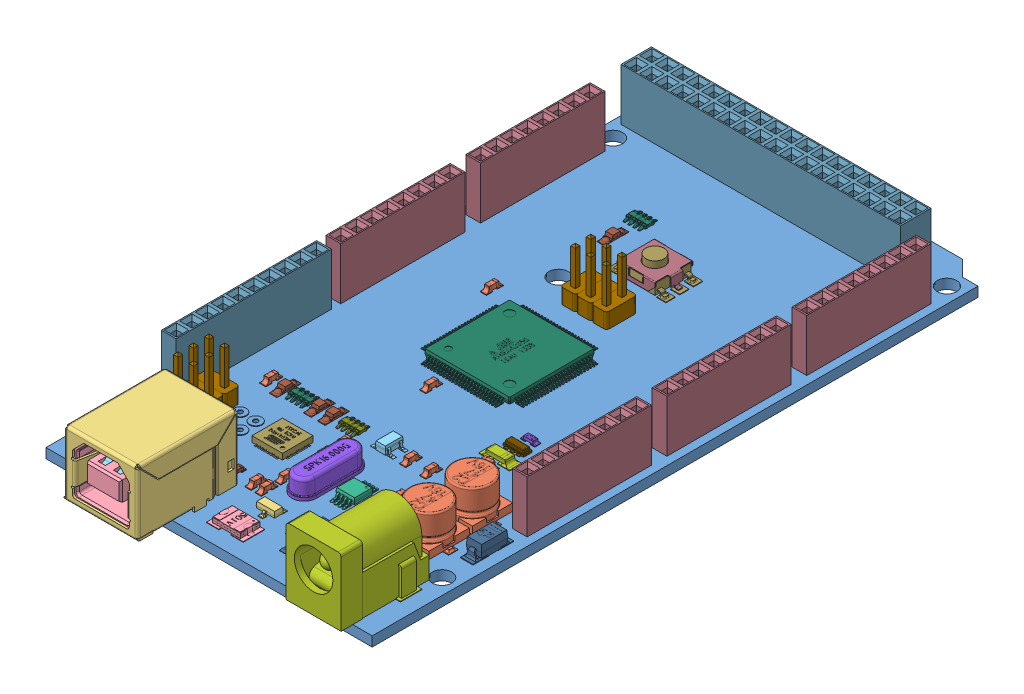
SolidWorks assembly arduino MEGA2650, configuration Default. Lengths in mm.
Overall size (53.34 15.25 107.95).
69 component instances, 33 part files, 170 mates.
Components (placement in the parent):
- MEGAboard-1: MEGAboard [Default] at origin size (53.34 1.6 101.6)
- 47uf CAP Dcase-1: 47uf CAP Dcase [Default] at (-9.144 0 -18.415) x (0 0 -1) z (1 0 0) size (6.6 5.81 8)
- USB type b-1: USB type b [Default] at (-38.02 0.43 6.35) size (13.72 15.2 16.5)
  - USB SHELL-1: USB SHELL [Default] at origin size (13.72 15.2 16.5)
  - USB core-1: USB core [Default] at origin size (11.3 10.68 15.75)
  - usb top contact-1: usb top contact [Default] at (1.25 6.09 -0.38) size (1 9.67 13.76)
  - usb btm contact-1: usb btm contact [Default] at (1.25 4.41 -0.38) size (1 6.84 11.76)
  - usb btm contact-2: usb btm contact [Default] at (-1.25 4.41 -0.38) size (1 6.84 11.76)
  - usb top contact-2: usb top contact [Default] at (-1.25 6.09 -0.38) size (1 9.67 13.76)
- power jack-1: power jack [Default] at (-7.675 0 1.905) size (11.2 15.2 15.9)
- 47uf CAP Dcase-2: 47uf CAP Dcase [Default] at (-9.144 0 -25.527) x (0 0 -1) z (1 0 0) size (6.6 5.81 8)
- crystal-1: crystal [Default] at (-26.035 0 -18.415) x (1 0 0) z (0 0 -1) size (4 5 11)
- 2pin_header__02-1: 2pin_header__02 [Default] at (-46.23 0 -15.75) size (5 11.75 2.54)
- reg-1: reg [Default] at (-17.78 0 -8.636) size (6.5 1.69 8.3)
- led-1: led [Default] at (-34.29 0 -27.94) x (0 0 1) z (-1 0 0) size (4 0.86 1.35)
- 2pin_header__02-2: 2pin_header__02 [Default] at (-30.43 0 -64.91) x (0 0 1) z (-1 0 0) size (5 11.75 2.54)
- 2pin_header__02-3: 2pin_header__02 [Default] at (-27.89 0 -64.91) x (0 0 1) z (-1 0 0) size (5 11.75 2.54)
- 2pin_header__02-4: 2pin_header__02 [Default] at (-25.35 0 -64.91) x (0 0 1) z (-1 0 0) size (5 11.75 2.54)
- 2pin_header__02-5: 2pin_header__02 [Default] at (-46.23 0 -18.29) size (5 11.75 2.54)
- 2pin_header__02-6: 2pin_header__02 [Default] at (-46.23 0 -20.83) size (5 11.75 2.54)
- atmega16u2-1: atmega16u2 [Default] at (-34.671 0.06 -20) x (1 0 0) z (0 0 -1) size (5.5 1.01 5.5)
- led-2: led [Default] at (-36.576 0 -27.94) x (0 0 -1) z (1 0 0) size (4 0.86 1.35)
- led-3: led [Default] at (-42.164 0 -27.94) x (0 0 1) z (-1 0 0) size (4 0.86 1.35)
- led-4: led [Default] at (-36.83 0 -76.2) x (0 0 1) z (-1 0 0) size (4 0.86 1.35)
- 8 PORT HEADER-3: 8 PORT HEADER [Default] at (-50.8 0 -45.72) x (0 0 -1) z (1 0 0) size (20.32 10.51 2.41)
- 8 PORT HEADER-4: 8 PORT HEADER [Default] at (-2.54 0 -27.94) x (0 0 -1) z (1 0 0) size (20.32 10.51 2.41)
- 8 PORT HEADER-6: 8 PORT HEADER [Default] at (-2.54 0 -50.8) x (0 0 -1) z (1 0 0) size (20.32 10.51 2.41)
- 10 PORT HEADER-1: 10 PORT HEADER [Default] at (-50.8 0 -18.796) x (0 0 -1) z (1 0 0) size (25.4 10.51 2.41)
- 102 RESISTOR PACK-1: 102 RESISTOR PACK [Default] at (-36.83 0 -80.645) size (3.2 0.46 3)
- 102 RESISTOR PACK-2: 102 RESISTOR PACK [Default] at (-39.37 0 -27.94) size (3.2 0.46 3)
- 103 RESISTOR PACK-3: 103 RESISTOR PACK [Default] at (-31.115 0 -27.94) size (3.2 0.46 3)
- 220 RESISTOR PACK-1: 220 RESISTOR PACK [Default] at (-37.084 0 -12.065) size (3.2 0.46 3)
- 16mhz crystal - measured-1: 16mhz crystal - measured [Default] at (-14.605 0 -38.354) size (3.4 0.8 2)
- PADS001-1: PADS001 [Default] at (-39.878 0.1 -18.288) x (-1 0 0) z (0 0 1) size (4.54 0.1 4.54)
- 603 cap on pad-1: 603 cap on pad [Default] at (-44.45 0 -27.94) x (0 0 -1) z (1 0 0) size (2.76 0.9 1.12)
- ssot3-1: ssot3 [Default] at (-25.908 0 -9.144) x (-1 0 0) z (0 0 -1) size (3 1.13 3.09)
- mf-msmf050-2-1: mf-msmf050-2 [Default] at (-26.67 0 -4.445) size (5.77 1.02 3.72)
- 603 cap on pad-2: 603 cap on pad [Default] at (-29.337 0 -24.765) x (0 0 1) z (-1 0 0) size (2.76 0.9 1.12)
- 603 cap on pad-3: 603 cap on pad [Default] at (-30.988 0 -12.065) x (0 0 -1) z (1 0 0) size (2.76 0.9 1.12)
- lmv358-1: lmv358 [Default] at (-25.146 0 -27.94) size (3.7 1.4 2.9)
- 603 cap on pad-4: 603 cap on pad [Default] at (-17.653 0 -14.351) size (2.76 0.9 1.12)
- 603 cap on pad-5: 603 cap on pad [Default] at (-29.337 0 -12.065) x (0 0 1) z (-1 0 0) size (2.76 0.9 1.12)
- 603 cap on pad-6: 603 cap on pad [Default] at (-29.337 0 -21.59) x (0 0 1) z (-1 0 0) size (2.76 0.9 1.12)
- 603 cap on pad-7: 603 cap on pad [Default] at (-29.337 0 -15.24) x (0 0 1) z (-1 0 0) size (2.76 0.9 1.12)
- 603 cap on pad-8: 603 cap on pad [Default] at (-42.291 0 -12.065) x (0 0 1) z (-1 0 0) size (2.76 0.9 1.12)
- lp2985dgkr-1: lp2985dgkr [Default] at (-21.336 0 -18.415) x (0 0 -1) z (1 0 0) size (5.85 1.1 3)
- cd1206 diode-1: cd1206 diode [Default] at (-14.605 0 -35.56) x (0 0 1) z (-1 0 0) size (2.07 0.96 5)
- cd1206 diode-2: cd1206 diode [Default] at (-46.228 0 -13.081) x (0 0 1) z (-1 0 0) size (2.07 0.96 5)
- 603 resistor-1: 603 resistor [Default] at (-29.337 0 -18.415) x (0 0 1) z (-1 0 0) size (2.36 0.61 1.03)
- blm21-1: blm21 [Default] at (-45.085 0 -8.255) x (0 0 -1) z (1 0 0) size (2.76 0.95 1.32)
- m7 diode-1: m7 diode [Default] at (-2.794 0 -21.59) x (0 0 -1) z (1 0 0) size (6.66 2.35 2.5)
- MLC0603-1: MLC0603 [Default] at (-34.29 0 -12.065) x (0 0 -1) z (1 0 0) size (2.36 0.6 1.03)
- MLC0603-2: MLC0603 [Default] at (-39.878 0 -12.065) x (0 0 -1) z (1 0 0) size (2.36 0.6 1.03)
- RESET BUTTON-1: RESET BUTTON [Default] at (-27.94 0 -74.168) x (0 0 -1) z (1 0 0) size (6.2 3.1 9.6)
  - RESET CORE-1: RESET CORE [Default] at (0 0.1 0) x (-1 0 0) z (0 0 -1) size (6.2 3.1 9.6)
  - RESET-1: RESET [Default] at (0 0.1 0) x (0 0 1) z (-1 0 0) size (7.3 2 6.2)
- 8 PORT HEADER-5: 8 PORT HEADER [Default] at (-2.54 0 -73.66) x (0 0 -1) z (1 0 0) size (20.32 10.51 2.41)
- 8 PORT HEADER-7: 8 PORT HEADER [Default] at (-50.8 0 -68.58) x (0 0 -1) z (1 0 0) size (20.32 10.51 2.41)
- 603 cap on pad-9: 603 cap on pad [Default] at (-21.59 0 -27.94) x (0 0 1) z (-1 0 0) size (2.76 0.9 1.12)
- 603 cap on pad-10: 603 cap on pad [Default] at (-18.288 0 -27.94) x (0 0 1) z (-1 0 0) size (2.76 0.9 1.12)
- 103 RESISTOR PACK-4: 103 RESISTOR PACK [Default] at (-16.51 0 -18.415) size (3.2 0.46 3)
- 603 cap on pad-11: 603 cap on pad [Default] at (-17.145 0 -21.59) x (0 0 -1) z (1 0 0) size (2.76 0.9 1.12)
- 603 cap on pad-12: 603 cap on pad [Default] at (-39.37 0 -58.928) x (0 0 1) z (-1 0 0) size (2.76 0.9 1.12)
- 603 cap on pad-13: 603 cap on pad [Default] at (-14.605 0 -33.528) size (2.76 0.9 1.12)
- 603 resistor-2: 603 resistor [Default] at (-14.605 0 -40.513) x (-1 0 0) z (0 0 -1) size (2.36 0.61 1.03)
- 603 cap on pad-14: 603 cap on pad [Default] at (-7.112 0 -38.608) x (0 0 1) z (-1 0 0) size (2.76 0.9 1.12)
- 603 cap on pad-15: 603 cap on pad [Default] at (-30.4038 0 -40.0558) x (0 0 1) z (-1 0 0) size (2.76 0.9 1.12)
- 18 X 2 ROW HEADER-1: 18 X 2 ROW HEADER [Default] at (-50.8 0 -95.25) size (45.72 10.51 4.95)
- atmega2650-16AU-1: atmega2650-16AU [Default] at (-28.3464 0.1 -50.8) x (0 0 1) z (-1 0 0) size (16.8 1.1 16.8)
Mates (geometry in assembly coordinates):
- Distance1: distance = 1.905 mm aligned: plane of power jack-1 through (-7.675 0 1.905) normal (0 0 1); plane of MEGAboard-1 through (0 0 0) normal (0 0 1)
- Coincident2: coincident aligned: plane of MEGAboard-1 through (0 0 0) normal (0 1 0); plane of power jack-1 through (-7.675 0 1.905) normal (0 1 0)
- Coincident3: coincident anti-aligned: plane of MEGAboard-1 through (0 0 0) normal (0 1 0); plane of USB type b-1/USB core-1 through (-38.02 0 6.35) normal (0 -1 0)
- Distance2: distance = 6.35 mm aligned: plane of USB type b-1/USB SHELL-1 through (-38.02 0.43 6.35) normal (0 0 1); plane of MEGAboard-1 through (0 0 0) normal (0 0 1)
- Coincident5: coincident aligned: plane of MEGAboard-1 through (0 0 0) normal (0 1 0); plane of 47uf CAP Dcase-1 through (-9.144 0 -18.415) normal (0 1 0)
- Parallel1: parallel anti-aligned: plane of MEGAboard-1 through (0 0 0) normal (0 0 1); plane of 47uf CAP Dcase-1 through (-9.144 0 -18.415) normal (0 0 -1)
- Coincident7: coincident aligned: plane of 47uf CAP Dcase-1 through (-5.844 1.5 -15.115) normal (1 0 0); plane of 47uf CAP Dcase-2 through (-5.844 1.5 -22.227) normal (1 0 0)
- Coincident8: coincident anti-aligned: plane of MEGAboard-1 through (0 0 0) normal (0 1 0); plane of 47uf CAP Dcase-2 through (-7.919 0 -25.527) normal (0 -1 0)
- Distance3: distance = 3.175 mm aligned: plane of power jack-1 through (-3.175 10.5 -1.595) normal (1 0 0); plane of MEGAboard-1 through (0 -1.6 0) normal (1 0 0)
- Distance4: distance = 32 mm aligned: plane of USB type b-1/USB SHELL-1 through (-32 0.43 6.35) normal (1 0 0); plane of MEGAboard-1 through (0 -1.6 0) normal (1 0 0)
- Coincident11: coincident anti-aligned: plane of MEGAboard-1 through (0 0 0) normal (0 1 0); plane of crystal-1 through (-26.035 0 -21.915) normal (0 -1 0)
- Concentric1: concentric aligned: cylinder of MEGAboard-1 through (-26.035 -10 -15.875) axis (0 1 0) radius 0.5; cylinder of crystal-1 through (-26.035 -2 -15.875) axis (0 1 0) radius 0.4
- Concentric2: concentric aligned: cylinder of MEGAboard-1 through (-26.035 -10 -20.955) axis (0 1 0) radius 0.5; cylinder of crystal-1 through (-26.035 -2 -20.955) axis (0 1 0) radius 0.4
- Coincident12: coincident anti-aligned: plane of MEGAboard-1 through (0 0 0) normal (0 1 0); plane of 2pin_header__02-1 through (-44.23 0 -14.98) normal (0 -1 0)
- Distance5: distance = 15.75 mm aligned: plane of 2pin_header__02-1 through (-46.23 0 -15.75) normal (0 0 1); plane of assembly through (0 0 0) normal (0 0 1)
- Distance6: distance = 46.23 mm aligned: plane of 2pin_header__02-1 through (-46.23 0 -15.75) normal (1 0 0); plane of assembly through (0 0 0) normal (1 0 0)
- Coincident15: coincident anti-aligned: plane of MEGAboard-1 through (0 0 0) normal (0 1 0); plane of 2pin_header__02-2 through (-31.2 0 -62.91) normal (0 -1 0)
- Distance7: distance = 64.91 mm aligned: plane of 2pin_header__02-2 through (-30.43 0 -64.91) normal (0 0 1); plane of assembly through (0 0 0) normal (0 0 1)
- Distance8: distance = 30.43 mm anti-aligned: plane of 2pin_header__02-2 through (-30.43 0 -64.91) normal (-1 0 0); plane of assembly through (0 0 0) normal (1 0 0)
- Coincident19: coincident anti-aligned: plane of MEGAboard-1 through (0 0 0) normal (0 1 0); plane of reg-1 through (-17.78 0 -8.636) normal (0 -1 0)
- Coincident21: coincident anti-aligned: plane of MEGAboard-1 through (0 0 0) normal (0 1 0); plane of atmega16u2-1 through (-34.671 0 -20) normal (0 -1 0)
- Distance10: distance = 20 mm anti-aligned: plane of atmega16u2-1 through (-34.671 0.06 -20) normal (0 0 -1); plane of MEGAboard-1 through (0 0 0) normal (0 0 1)
- Distance11: distance = 34.671 mm aligned: plane of atmega16u2-1 through (-34.671 0.06 -20) normal (1 0 0); plane of MEGAboard-1 through (0 0 0) normal (1 0 0)
- Coincident25: coincident anti-aligned: plane of MEGAboard-1 through (0 0 0) normal (0 1 0); plane of led-1 through (-34.29 0 -28.94) normal (0 -1 0)
- Distance12: distance = 34.29 mm anti-aligned: plane of led-1 through (-34.29 0 -27.94) normal (-1 0 0); plane of MEGAboard-1 through (0 0 0) normal (1 0 0)
- Distance13: distance = 27.94 mm aligned: plane of led-1 through (-34.29 0 -27.94) normal (0 0 1); plane of MEGAboard-1 through (0 0 0) normal (0 0 1)
- Coincident28: coincident aligned: plane of led-2 through (-36.576 0 -26.94) normal (0 -1 0); plane of led-3 through (-42.164 0 -28.94) normal (0 -1 0)
- Coincident29: coincident anti-aligned: plane of led-1 through (-34.29 0 -27.94) normal (0 0 1); plane of led-2 through (-36.576 0 -27.94) normal (0 0 -1)
- Coincident30: coincident aligned: plane of led-1 through (-34.29 0 -27.94) normal (0 0 1); plane of led-3 through (-42.164 0 -27.94) normal (0 0 1)
- Distance14: distance = 36.576 mm aligned: plane of led-2 through (-36.576 0 -27.94) normal (1 0 0); plane of MEGAboard-1 through (0 0 0) normal (1 0 0)
- Coincident32: coincident anti-aligned: plane of MEGAboard-1 through (0 0 0) normal (0 1 0); plane of led-2 through (-36.576 0 -26.94) normal (0 -1 0)
- Distance15: distance = 42.164 mm anti-aligned: plane of led-3 through (-42.164 0 -27.94) normal (-1 0 0); plane of MEGAboard-1 through (0 0 0) normal (1 0 0)
- Coincident34: coincident anti-aligned: plane of MEGAboard-1 through (0 0 0) normal (0 1 0); plane of led-4 through (-36.83 0 -77.2) normal (0 -1 0)
- Distance16: distance = 36.83 mm anti-aligned: plane of led-4 through (-36.83 0 -76.2) normal (-1 0 0); plane of MEGAboard-1 through (0 0 0) normal (1 0 0)
- Distance17: distance = 76.2 mm aligned: plane of led-4 through (-36.83 0 -76.2) normal (0 0 1); plane of MEGAboard-1 through (0 0 0) normal (0 0 1)
- Coincident37: coincident aligned: plane of MEGAboard-1 through (0 0 0) normal (0 1 0); plane of 8 PORT HEADER-4 through (-2.54 0 -27.94) normal (0 1 0)
- Coincident38: coincident aligned: plane of MEGAboard-1 through (0 0 0) normal (0 1 0); plane of 8 PORT HEADER-3 through (-50.8 0 -45.72) normal (0 1 0)
- Parallel2: parallel aligned: plane of MEGAboard-1 through (0 0 0) normal (1 0 0); plane of 8 PORT HEADER-4 through (-2.54 0 -27.94) normal (1 0 0)
- Parallel3: parallel aligned: plane of MEGAboard-1 through (0 0 0) normal (1 0 0); plane of 8 PORT HEADER-3 through (-50.8 0 -45.72) normal (1 0 0)
- Concentric5: concentric aligned: cylinder of MEGAboard-1 through (-2.54 -1.65 -27.94) axis (0 1 0) radius 0.4; line of 8 PORT HEADER-4 through (-2.54 -2.5255 -27.94) axis (0 1 0)
- Concentric6: concentric aligned: cylinder of MEGAboard-1 through (-50.8 -1.65 -45.72) axis (0 1 0) radius 0.4; line of 8 PORT HEADER-3 through (-50.8 -2.5255 -45.72) axis (0 1 0)
- Coincident43: coincident aligned: plane of MEGAboard-1 through (0 0 0) normal (0 1 0); plane of 10 PORT HEADER-1 through (-50.8 0 -18.796) normal (0 1 0)
- Coincident44: coincident aligned: plane of MEGAboard-1 through (0 0 0) normal (0 1 0); plane of 8 PORT HEADER-6 through (-2.54 0 -50.8) normal (0 1 0)
- Parallel4: parallel aligned: plane of MEGAboard-1 through (0 0 0) normal (1 0 0); plane of 8 PORT HEADER-6 through (-2.54 0 -50.8) normal (1 0 0)
- Parallel5: parallel aligned: plane of MEGAboard-1 through (0 0 0) normal (1 0 0); plane of 10 PORT HEADER-1 through (-50.8 0 -18.796) normal (1 0 0)
- Concentric7: concentric aligned: cylinder of MEGAboard-1 through (-50.8 -1.65 -18.796) axis (0 1 0) radius 0.4; line of 10 PORT HEADER-1 through (-50.8 -2.5255 -18.796) axis (0 1 0)
- Concentric9: concentric aligned: cylinder of MEGAboard-1 through (-2.54 -1.65 -50.8) axis (0 1 0) radius 0.4; line of 8 PORT HEADER-6 through (-2.54 -2.5255 -50.8) axis (0 1 0)
- Distance18: distance = 8.636 mm: plane of reg-1 through (-17.78 0 -8.636) normal (0 0 1); line of MEGAboard-1 through (0 53.34 -53.34) axis (0 0 1)
- Distance19: distance = 17.78 mm aligned: plane of reg-1 through (-17.78 0 -8.636) normal (1 0 0); plane of MEGAboard-1 through (0 0 0) normal (1 0 0)
- Coincident55: coincident anti-aligned: plane of MEGAboard-1 through (0 0 0) normal (0 1 0); plane of 102 RESISTOR PACK-1 through (-37.03 0 -81.345) normal (0 -1 0)
- Distance20: distance = 36.83 mm aligned: plane of 102 RESISTOR PACK-1 through (-36.83 0 -80.645) normal (1 0 0); plane of MEGAboard-1 through (0 0 0) normal (1 0 0)
- Distance21: distance = 80.645 mm aligned: plane of 102 RESISTOR PACK-1 through (-36.83 0 -80.645) normal (0 0 1); plane of MEGAboard-1 through (0 0 0) normal (0 0 1)
- Coincident58: coincident aligned: plane of 102 RESISTOR PACK-2 through (-39.37 0 -27.94) normal (0 1 0); plane of 103 RESISTOR PACK-3 through (-31.115 0 -27.94) normal (0 1 0)
- Coincident59: coincident aligned: plane of MEGAboard-1 through (0 0 0) normal (0 1 0); plane of 103 RESISTOR PACK-3 through (-31.115 0 -27.94) normal (0 1 0)
- Coincident60: coincident aligned: plane of 102 RESISTOR PACK-2 through (-39.37 0 -27.94) normal (0 0 1); plane of 103 RESISTOR PACK-3 through (-31.115 0 -27.94) normal (0 0 1)
- Distance22: distance = 31.115 mm aligned: plane of 103 RESISTOR PACK-3 through (-31.115 0 -27.94) normal (1 0 0); plane of MEGAboard-1 through (0 0 0) normal (1 0 0)
- Distance23: distance = 39.37 mm aligned: plane of 102 RESISTOR PACK-2 through (-39.37 0 -27.94) normal (1 0 0); plane of MEGAboard-1 through (0 0 0) normal (1 0 0)
- Distance24: distance = 27.94 mm aligned: plane of 102 RESISTOR PACK-2 through (-39.37 0 -27.94) normal (0 0 1); plane of MEGAboard-1 through (0 0 0) normal (0 0 1)
- Distance25: distance = 12.065 mm aligned: plane of 220 RESISTOR PACK-1 through (-37.084 0 -12.065) normal (0 0 1); plane of MEGAboard-1 through (0 0 0) normal (0 0 1)
- Distance26: distance = 37.084 mm aligned: plane of 220 RESISTOR PACK-1 through (-37.084 0 -12.065) normal (1 0 0); plane of MEGAboard-1 through (0 0 0) normal (1 0 0)
- Coincident66: coincident aligned: plane of MEGAboard-1 through (0 0 0) normal (0 1 0); plane of 220 RESISTOR PACK-1 through (-37.084 0 -12.065) normal (0 1 0)
- Coincident67: coincident anti-aligned: plane of MEGAboard-1 through (0 0 0) normal (0 1 0); plane of 16mhz crystal - measured-1 through (-14.605 0 -38.354) normal (0 -1 0)
- Distance27: distance = 14.605 mm aligned: plane of 16mhz crystal - measured-1 through (-14.605 0 -38.354) normal (1 0 0); plane of MEGAboard-1 through (0 0 0) normal (1 0 0)
- Distance28: distance = 38.354 mm aligned: plane of 16mhz crystal - measured-1 through (-14.605 0 -38.354) normal (0 0 1); plane of MEGAboard-1 through (0 0 0) normal (0 0 1)
- Coincident70: coincident anti-aligned: plane of MEGAboard-1 through (0 0 0) normal (0 1 0); plane of PADS001-1 through (-42.418 0 -18.288) normal (0 -1 0)
- Distance29: distance = 18.288 mm aligned: plane of PADS001-1 through (-39.878 0.1 -18.288) normal (0 0 1); plane of MEGAboard-1 through (0 0 0) normal (0 0 1)
- Distance30: distance = 39.878 mm anti-aligned: plane of PADS001-1 through (-39.878 0.1 -18.288) normal (-1 0 0); plane of MEGAboard-1 through (0 0 0) normal (1 0 0)
- Distance31: distance = 4.445 mm aligned: plane of mf-msmf050-2-1 through (-26.67 0 -4.445) normal (0 0 1); plane of MEGAboard-1 through (0 0 0) normal (0 0 1)
- Distance32: distance = 26.67 mm aligned: plane of mf-msmf050-2-1 through (-26.67 0 -4.445) normal (1 0 0); plane of MEGAboard-1 through (0 0 0) normal (1 0 0)
- Coincident72: coincident aligned: plane of MEGAboard-1 through (0 0 0) normal (0 1 0); plane of mf-msmf050-2-1 through (-26.67 0 -4.445) normal (0 1 0)
- Distance33: distance = 9.144 mm anti-aligned: plane of MEGAboard-1 through (0 0 0) normal (0 0 1); plane of ssot3-1 through (-25.908 0 -9.144) normal (0 0 -1)
- Distance78: distance = 0.762 mm anti-aligned: plane of ssot3-1 through (-25.908 0 -9.144) normal (-1 0 0); plane of mf-msmf050-2-1 through (-26.67 0 -4.445) normal (1 0 0)
- Coincident75: coincident aligned: plane of MEGAboard-1 through (0 0 0) normal (0 1 0); plane of ssot3-1 through (-25.908 0 -9.144) normal (0 1 0)
- Coincident76: coincident anti-aligned: plane of led-1 through (-34.29 0 -27.94) normal (0 0 1); plane of 603 cap on pad-1 through (-44.45 0 -27.94) normal (0 0 -1)
- Coincident77: coincident aligned: plane of MEGAboard-1 through (0 0 0) normal (0 1 0); plane of 603 cap on pad-1 through (-44.45 0 -27.94) normal (0 1 0)
- Distance34: distance = 44.45 mm aligned: plane of 603 cap on pad-1 through (-44.45 0 -27.94) normal (1 0 0); plane of MEGAboard-1 through (0 0 0) normal (1 0 0)
- Coincident79: coincident aligned: plane of 603 cap on pad-2 through (-29.337 0 -24.765) normal (0 1 0); plane of 603 cap on pad-3 through (-30.988 0 -12.065) normal (0 1 0)
- Coincident81: coincident aligned: plane of MEGAboard-1 through (0 0 0) normal (0 1 0); plane of 603 cap on pad-2 through (-29.337 0 -24.765) normal (0 1 0)
- Distance65: distance = 24.765 mm aligned: plane of 603 cap on pad-2 through (-29.337 0 -24.765) normal (0 0 1); plane of MEGAboard-1 through (0 0 0) normal (0 0 1)
- Distance36: distance = 29.337 mm anti-aligned: plane of 603 cap on pad-2 through (-29.337 0 -24.765) normal (-1 0 0); plane of MEGAboard-1 through (0 0 0) normal (1 0 0)
- Distance37: distance = 30.988 mm aligned: plane of 603 cap on pad-3 through (-30.988 0 -12.065) normal (1 0 0); plane of MEGAboard-1 through (0 0 0) normal (1 0 0)
- Distance38: distance = 27.94 mm aligned: plane of MEGAboard-1 through (0 0 0) normal (0 0 1); plane of lmv358-1 through (-25.146 0 -27.94) normal (0 0 1)
- Distance39: distance = 21.971 mm anti-aligned: plane of lmv358-1 through (-25.146 0 -27.94) normal (1 0 0); plane of MEGAboard-1 through (0 0 0) normal (0 0 1)
- Coincident88: coincident aligned: plane of MEGAboard-1 through (0 0 0) normal (0 1 0); plane of lmv358-1 through (-25.146 0 -27.94) normal (0 1 0)
- Distance40: distance = 14.351 mm aligned: plane of 603 cap on pad-4 through (-17.653 0 -14.351) normal (0 0 1); plane of MEGAboard-1 through (0 0 0) normal (0 0 1)
- Distance41: distance = 17.653 mm aligned: plane of 603 cap on pad-4 through (-17.653 0 -14.351) normal (1 0 0); plane of MEGAboard-1 through (0 0 0) normal (1 0 0)
- Coincident91: coincident aligned: plane of MEGAboard-1 through (0 0 0) normal (0 1 0); plane of 603 cap on pad-4 through (-17.653 0 -14.351) normal (0 1 0)
- Coincident92: coincident aligned: plane of MEGAboard-1 through (0 0 0) normal (0 1 0); plane of 603 cap on pad-7 through (-29.337 0 -15.24) normal (0 1 0)
- Coincident93: coincident aligned: plane of MEGAboard-1 through (0 0 0) normal (0 1 0); plane of 603 cap on pad-6 through (-29.337 0 -21.59) normal (0 1 0)
- Coincident94: coincident aligned: plane of 603 cap on pad-5 through (-29.337 0 -12.065) normal (0 1 0); plane of MEGAboard-1 through (0 0 0) normal (0 1 0)
- Coincident95: coincident aligned: plane of 603 cap on pad-8 through (-42.291 0 -12.065) normal (0 1 0); plane of MEGAboard-1 through (0 0 0) normal (0 1 0)
- Coincident96: coincident aligned: plane of 603 cap on pad-7 through (-29.337 0 -15.24) normal (-1 0 0); plane of 603 cap on pad-6 through (-29.337 0 -21.59) normal (-1 0 0)
- Distance42: distance = 29.337 mm anti-aligned: plane of 603 cap on pad-7 through (-29.337 0 -15.24) normal (-1 0 0); plane of MEGAboard-1 through (0 0 0) normal (1 0 0)
- Distance43: distance = 21.59 mm: plane of 603 cap on pad-6 through (-29.337 0 -21.59) normal (0 0 1); line of MEGAboard-1 through (0 53.34 -53.34) axis (0 0 1)
- Distance44: distance = 15.24 mm aligned: plane of 603 cap on pad-7 through (-29.337 0 -15.24) normal (0 0 1); plane of MEGAboard-1 through (0 0 0) normal (0 0 1)
- Distance45: distance = 29.337 mm anti-aligned: plane of 603 cap on pad-5 through (-29.337 0 -12.065) normal (-1 0 0); plane of MEGAboard-1 through (0 0 0) normal (1 0 0)
- Distance46: distance = 12.065 mm aligned: plane of 603 cap on pad-5 through (-29.337 0 -12.065) normal (0 0 1); plane of MEGAboard-1 through (0 0 0) normal (0 0 1)
- Distance47: distance = 42.291 mm anti-aligned: plane of 603 cap on pad-8 through (-42.291 0 -12.065) normal (-1 0 0); plane of MEGAboard-1 through (0 0 0) normal (1 0 0)
- Distance48: distance = 12.065 mm aligned: plane of 603 cap on pad-8 through (-42.291 0 -12.065) normal (0 0 1); plane of MEGAboard-1 through (0 0 0) normal (0 0 1)
- Distance49: distance = 21.336 mm aligned: plane of lp2985dgkr-1 through (-21.336 0 -18.415) normal (1 0 0); plane of MEGAboard-1 through (0 0 0) normal (1 0 0)
- Distance50: distance = 18.415 mm anti-aligned: plane of lp2985dgkr-1 through (-21.336 0 -18.415) normal (0 0 -1); plane of MEGAboard-1 through (0 0 0) normal (0 0 1)
- Coincident99: coincident aligned: plane of MEGAboard-1 through (0 0 0) normal (0 1 0); plane of lp2985dgkr-1 through (-21.336 0 -18.415) normal (0 1 0)
- Distance51: distance = 14.605 mm anti-aligned: plane of cd1206 diode-1 through (-14.605 0 -35.56) normal (-1 0 0); plane of MEGAboard-1 through (0 0 0) normal (1 0 0)
- Distance52: distance = 35.56 mm aligned: plane of cd1206 diode-1 through (-14.605 0 -35.56) normal (0 0 1); plane of MEGAboard-1 through (0 0 0) normal (0 0 1)
- Coincident102: coincident aligned: plane of MEGAboard-1 through (0 0 0) normal (0 1 0); plane of cd1206 diode-1 through (-14.605 0 -35.56) normal (0 1 0)
- Distance53: distance = 46.228 mm anti-aligned: plane of cd1206 diode-2 through (-46.228 0 -13.081) normal (-1 0 0); plane of MEGAboard-1 through (0 0 0) normal (1 0 0)
- Distance54: distance = 13.081 mm aligned: plane of MEGAboard-1 through (0 0 0) normal (0 0 1); plane of cd1206 diode-2 through (-46.228 0 -13.081) normal (0 0 1)
- Coincident105: coincident aligned: plane of MEGAboard-1 through (0 0 0) normal (0 1 0); plane of cd1206 diode-2 through (-46.228 0 -13.081) normal (0 1 0)
- Distance55: distance = 29.337 mm anti-aligned: plane of 603 resistor-1 through (-29.337 0 -18.415) normal (-1 0 0); plane of MEGAboard-1 through (0 0 0) normal (1 0 0)
- Distance56: distance = 18.415 mm aligned: plane of 603 resistor-1 through (-29.337 0 -18.415) normal (0 0 1); plane of MEGAboard-1 through (0 0 0) normal (0 0 1)
- Coincident108: coincident aligned: plane of MEGAboard-1 through (0 0 0) normal (0 1 0); plane of 603 resistor-1 through (-29.337 0 -18.415) normal (0 1 0)
- Distance57: distance = 8.255 mm anti-aligned: plane of blm21-1 through (-45.085 0 -8.255) normal (0 0 -1); plane of MEGAboard-1 through (0 0 0) normal (0 0 1)
- Distance58: distance = 45.085 mm aligned: plane of blm21-1 through (-45.085 0 -8.255) normal (1 0 0); plane of MEGAboard-1 through (0 0 0) normal (1 0 0)
- Distance59: distance = 21.59 mm anti-aligned: plane of m7 diode-1 through (-2.794 0 -21.59) normal (0 0 -1); plane of MEGAboard-1 through (0 0 0) normal (0 0 1)
- Distance60: distance = 2.794 mm aligned: plane of m7 diode-1 through (-2.794 0 -21.59) normal (1 0 0); plane of MEGAboard-1 through (0 0 0) normal (1 0 0)
- Coincident113: coincident aligned: plane of MEGAboard-1 through (0 0 0) normal (0 1 0); plane of m7 diode-1 through (-2.794 0 -21.59) normal (0 1 0)
- Coincident114: coincident anti-aligned: plane of 220 RESISTOR PACK-1 through (-37.084 0 -12.065) normal (0 0 1); plane of MLC0603-1 through (-34.29 0 -12.065) normal (0 0 -1)
- Distance61: distance = 34.29 mm aligned: plane of MLC0603-1 through (-34.29 0 -12.065) normal (1 0 0); plane of MEGAboard-1 through (0 0 0) normal (1 0 0)
- Coincident115: coincident aligned: plane of MEGAboard-1 through (0 0 0) normal (0 1 0); plane of MLC0603-1 through (-34.29 0 -12.065) normal (0 1 0)
- Coincident116: coincident aligned: plane of MEGAboard-1 through (0 0 0) normal (0 1 0); plane of blm21-1 through (-45.085 0 -8.255) normal (0 1 0)
- Coincident117: coincident anti-aligned: plane of 220 RESISTOR PACK-1 through (-37.084 0 -12.065) normal (0 0 1); plane of MLC0603-2 through (-39.878 0 -12.065) normal (0 0 -1)
- Coincident118: coincident aligned: plane of MEGAboard-1 through (0 0 0) normal (0 1 0); plane of MLC0603-2 through (-39.878 0 -12.065) normal (0 1 0)
- Distance62: distance = 39.878 mm aligned: plane of MLC0603-2 through (-39.878 0 -12.065) normal (1 0 0); plane of MEGAboard-1 through (0 0 0) normal (1 0 0)
- Coincident122: coincident aligned: plane of MEGAboard-1 through (0 0 0) normal (0 1 0); plane of RESET BUTTON-1 through (-27.94 0 -74.168) normal (0 1 0)
- Concentric10: concentric aligned: cylinder of MEGAboard-1 through (-2.54 -1.65 -73.66) axis (0 1 0) radius 0.4; line of 8 PORT HEADER-5 through (-2.54 -2.5255 -73.66) axis (0 1 0)
- Coincident124: coincident anti-aligned: plane of MEGAboard-1 through (0 0 0) normal (0 1 0); plane of 8 PORT HEADER-5 through (-2.54 0 -73.66) normal (0 -1 0)
- Parallel6: parallel aligned: plane of MEGAboard-1 through (0 0 0) normal (1 0 0); plane of 8 PORT HEADER-5 through (-1.335 8.51 -72.39) normal (1 0 0)
- Concentric11: concentric aligned: cylinder of MEGAboard-1 through (-50.8 -1.65 -68.58) axis (0 1 0) radius 0.4; line of 8 PORT HEADER-7 through (-50.8 -2.5255 -68.58) axis (0 1 0)
- Parallel7: parallel aligned: plane of MEGAboard-1 through (0 0 0) normal (1 0 0); plane of 8 PORT HEADER-7 through (-49.595 8.51 -67.31) normal (1 0 0)
- Coincident128: coincident anti-aligned: plane of MEGAboard-1 through (0 0 0) normal (0 1 0); plane of 8 PORT HEADER-7 through (-50.8 0 -68.58) normal (0 -1 0)
- Distance63: distance = 27.94 mm aligned: plane of RESET BUTTON-1; plane of MEGAboard-1 through (0 0 0) normal (1 0 0)
- Distance64: distance = 74.168 mm anti-aligned: plane of RESET BUTTON-1 through (-27.94 0 -74.168) normal (0 0 -1); plane of MEGAboard-1 through (0 0 0) normal (0 0 1)
- Coincident131: coincident anti-aligned: plane of 603 cap on pad-3 through (-30.988 0 -12.065) normal (0 0 -1); plane of 603 cap on pad-5 through (-29.337 0 -12.065) normal (0 0 1)
- Distance66: distance = 25.146 mm aligned: plane of lmv358-1 through (-25.146 0 -27.94) normal (1 0 0); plane of MEGAboard-1 through (0 0 0) normal (1 0 0)
- Distance67: distance = 9.144 mm aligned: plane of 47uf CAP Dcase-2 through (-9.144 0 -25.527) normal (1 0 0); plane of MEGAboard-1 through (0 0 0) normal (1 0 0)
- Distance68: distance = 25.527 mm anti-aligned: plane of 47uf CAP Dcase-2 through (-9.144 0 -25.527) normal (0 0 -1); plane of MEGAboard-1 through (0 0 0) normal (0 0 1)
- Distance69: distance = 18.415 mm anti-aligned: plane of 47uf CAP Dcase-1 through (-9.144 0 -18.415) normal (0 0 -1); plane of MEGAboard-1 through (0 0 0) normal (0 0 1)
- Coincident136: coincident aligned: plane of 603 cap on pad-9 through (-21.59 0 -27.94) normal (0 0 1); plane of 603 cap on pad-10 through (-18.288 0 -27.94) normal (0 0 1)
- Distance72: distance = 3.302 mm aligned: plane of 603 cap on pad-9 through (-21.59 0 -27.94) normal (-1 0 0); plane of 603 cap on pad-10 through (-18.288 0 -27.94) normal (-1 0 0)
- Coincident143: coincident aligned: plane of 603 cap on pad-9 through (-21.59 0 -27.94) normal (0 1 0); plane of 603 cap on pad-10 through (-18.288 0 -27.94) normal (0 1 0)
- Coincident144: coincident aligned: plane of MEGAboard-1 through (0 0 0) normal (0 1 0); plane of 603 cap on pad-9 through (-21.59 0 -27.94) normal (0 1 0)
- Coincident145: coincident anti-aligned: plane of 603 cap on pad-1 through (-44.45 0 -27.94) normal (0 0 -1); plane of 603 cap on pad-9 through (-21.59 0 -27.94) normal (0 0 1)
- Distance73: distance = 21.59 mm anti-aligned: plane of 603 cap on pad-9 through (-21.59 0 -27.94) normal (-1 0 0); plane of MEGAboard-1 through (0 0 0) normal (1 0 0)
- Coincident147: coincident aligned: plane of MEGAboard-1 through (0 0 0) normal (0 1 0); plane of 103 RESISTOR PACK-4 through (-16.51 0 -18.415) normal (0 1 0)
- Distance74: distance = 16.51 mm aligned: plane of 103 RESISTOR PACK-4 through (-16.51 0 -18.415) normal (1 0 0); plane of MEGAboard-1 through (0 0 0) normal (1 0 0)
- Distance75: distance = 18.415 mm aligned: plane of 103 RESISTOR PACK-4 through (-16.51 0 -18.415) normal (0 0 1); plane of MEGAboard-1 through (0 0 0) normal (0 0 1)
- Coincident150: coincident aligned: plane of MEGAboard-1 through (0 0 0) normal (0 1 0); plane of 603 cap on pad-11 through (-17.145 0 -21.59) normal (0 1 0)
- Distance76: distance = 17.145 mm aligned: plane of 603 cap on pad-11 through (-17.145 0 -21.59) normal (1 0 0); plane of MEGAboard-1 through (0 0 0) normal (1 0 0)
- Distance77: distance = 21.59 mm anti-aligned: plane of 603 cap on pad-11 through (-17.145 0 -21.59) normal (0 0 -1); plane of MEGAboard-1 through (0 0 0) normal (0 0 1)
- Coincident154: coincident aligned: plane of MEGAboard-1 through (0 0 0) normal (0 1 0); plane of 603 cap on pad-12 through (-39.37 0 -58.928) normal (0 1 0)
- Distance79: distance = 39.37 mm anti-aligned: plane of 603 cap on pad-12 through (-39.37 0 -58.928) normal (-1 0 0); plane of MEGAboard-1 through (0 0 0) normal (1 0 0)
- Distance80: distance = 58.928 mm aligned: plane of 603 cap on pad-12 through (-39.37 0 -58.928) normal (0 0 1); plane of MEGAboard-1 through (0 0 0) normal (0 0 1)
- Coincident155: coincident aligned: plane of 603 cap on pad-13 through (-14.605 0 -33.528) normal (0 1 0); plane of 603 resistor-2 through (-14.605 0 -40.513) normal (0 1 0)
- Coincident156: coincident anti-aligned: plane of 603 cap on pad-13 through (-14.605 0 -33.528) normal (1 0 0); plane of 603 resistor-2 through (-14.605 0 -40.513) normal (-1 0 0)
- Distance81: distance = 6.985 mm anti-aligned: plane of 603 cap on pad-13 through (-14.605 0 -33.528) normal (0 0 1); plane of 603 resistor-2 through (-14.605 0 -40.513) normal (0 0 -1)
- Distance82: distance = 33.528 mm aligned: plane of 603 cap on pad-13 through (-14.605 0 -33.528) normal (0 0 1); plane of MEGAboard-1 through (0 0 0) normal (0 0 1)
- Distance83: distance = 14.605 mm aligned: plane of 603 cap on pad-13 through (-14.605 0 -33.528) normal (1 0 0); plane of MEGAboard-1 through (0 0 0) normal (1 0 0)
- Coincident160: coincident aligned: plane of MEGAboard-1 through (0 0 0) normal (0 1 0); plane of 603 resistor-2 through (-14.605 0 -40.513) normal (0 1 0)
- Coincident161: coincident aligned: plane of MEGAboard-1 through (0 0 0) normal (0 1 0); plane of 603 cap on pad-14 through (-7.112 0 -38.608) normal (0 1 0)
- Distance84: distance = 7.112 mm anti-aligned: plane of 603 cap on pad-14 through (-7.112 0 -38.608) normal (-1 0 0); plane of MEGAboard-1 through (0 0 0) normal (1 0 0)
- Distance85: distance = 38.608 mm aligned: plane of 603 cap on pad-14 through (-7.112 0 -38.608) normal (0 0 1); plane of MEGAboard-1 through (0 0 0) normal (0 0 1)
- Coincident164: coincident aligned: plane of MEGAboard-1 through (0 0 0) normal (0 1 0); plane of 603 cap on pad-15 through (-30.4038 0 -40.0558) normal (0 1 0)
- Distance86: distance = 30.4038 mm anti-aligned: plane of 603 cap on pad-15 through (-30.4038 0 -40.0558) normal (-1 0 0); plane of MEGAboard-1 through (0 0 0) normal (1 0 0)
- Distance87: distance = 40.0558 mm aligned: plane of 603 cap on pad-15 through (-30.4038 0 -40.0558) normal (0 0 1); plane of MEGAboard-1 through (0 0 0) normal (0 0 1)
- Concentric12: concentric anti-aligned: cylinder of MEGAboard-1 through (-50.8 -10 -96.52) axis (0 1 0) radius 0.4; cylinder of 18 X 2 ROW HEADER-1 through (-50.8 -1.55 -96.52) axis (0 -1 0) radius 0.75
- Parallel8: parallel anti-aligned: plane of MEGAboard-1 through (0 0 0) normal (0 0 1); plane of 18 X 2 ROW HEADER-1 through (-52.07 8.51 -97.725) normal (0 0 -1)
- Coincident169: coincident anti-aligned: plane of MEGAboard-1 through (0 0 0) normal (0 1 0); plane of 18 X 2 ROW HEADER-1 through (-50.8 0 -95.25) normal (0 -1 0)
- Distance88: distance = 50.8 mm aligned: plane of MEGAboard-1 through (0 0 0) normal (0 0 1); plane of atmega2650-16AU-1 through (-28.3464 0.1 -50.8) normal (0 0 1)
- Distance89: distance = 28.3464 mm anti-aligned: plane of atmega2650-16AU-1 through (-28.3464 0.1 -50.8) normal (-1 0 0); plane of MEGAboard-1 through (0 0 0) normal (1 0 0)
- Coincident172: coincident anti-aligned: plane of MEGAboard-1 through (0 0 0) normal (0 1 0); plane of atmega2650-16AU-1 through (-35.3464 0 -49.15) normal (0 -1 0)
